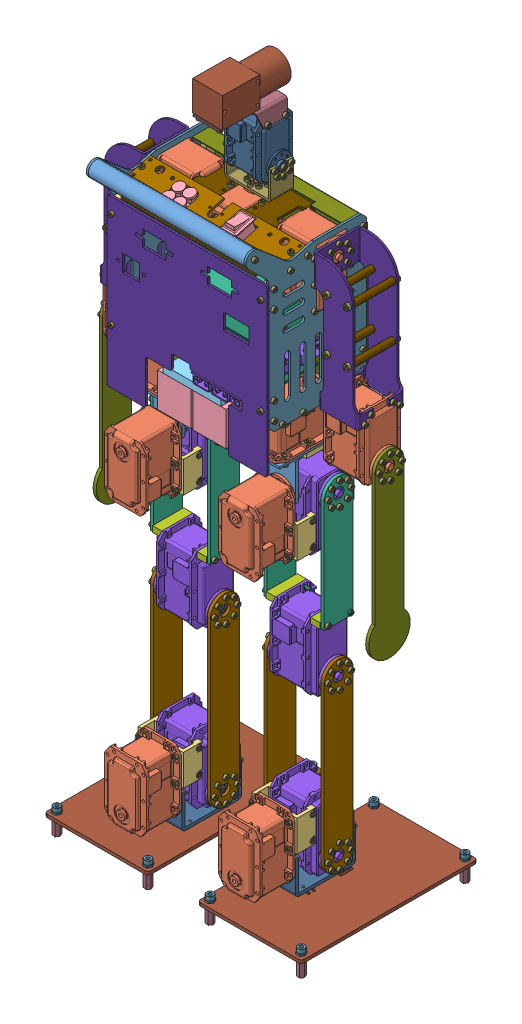
SolidWorks assembly 机器人, configuration 默认. Lengths in mm.
Overall size (525.52 712.77 348.31).
534 component instances, 40 part files, 172 mates.
Components (placement in the parent):
- 右腿-1: 右腿 [默认] at (1333.6429 -132.4302 49.3314) x (0.483512 -0.009844 -0.875282) z (0.842178 0.277849 0.4621) size (197.18 411.3 221.34)
  - 机器人-髋关节连接件-1: 机器人-髋关节连接件 [默认] at (-136.5981 582.4586 -53.7343) x (-0.483512 0.238647 -0.842178) z (-0.875282 -0.142634 0.4621) size (28 38.4 160)
  - MX64-1: MX64 [默认] at (-177.0712 253.729 -123.6615) x (0.483512 -0.238647 0.842178) z (0.875282 0.142634 -0.4621) size (40.2 62.1 50)
  - 机器人-舵机组合件-1: 机器人-舵机组合件 [默认] at (-152.084 293.2165 -100.9324) x (-0.483512 0.238647 -0.842178) z (0.009844 -0.960574 -0.277849) size (7.3 18.5 30)
  - 机器人-舵机组合件-2: 机器人-舵机组合件 [默认] at (-172.8697 274.8043 -145.9868) x (0.483512 -0.238647 0.842178) z (-0.009844 0.960574 0.277849) size (7.3 18.5 30)
  - 机器人-舵盘连接件-1: 机器人-舵盘连接件 [默认] at (-112.2264 257.0796 -159.9407) x (0.483512 -0.238647 0.842178) z (-0.009844 0.960574 0.277849) size (40 11.9 29)
  - MX64虚舵盘-1: MX64虚舵盘 [默认] at (-111.5044 237.7188 -167.2282) x (0.4798 -0.375849 0.792798) z (0.0606 0.915638 0.39741) size (28 4.56 28)
  - 机器人-上腿骨-1: 机器人-上腿骨 [默认] at (-150.3146 558.6458 -87.0655) x (0.483512 -0.238647 0.842178) z (0.875282 0.142634 -0.4621) size (3 122 28)
  - 机器人-上腿骨-2: 机器人-上腿骨 [默认] at (-123.7118 545.5154 -40.7289) x (0.483512 -0.238647 0.842178) z (0.875282 0.142634 -0.4621) size (3 122 28)
  - 机器人-腿骨支撑件-1: 机器人-腿骨支撑件 [默认] at (-147.8304 457.0695 -113.7131) x (0.875282 0.142634 -0.4621) z (0.483512 -0.238647 0.842178) size (30 5.6 9.01)
  - 机器人-腿骨支撑件-2: 机器人-腿骨支撑件 [默认] at (-127.0346 446.8053 -77.491) x (0.875282 0.142634 -0.4621) z (0.483512 -0.238647 0.842178) size (30 5.6 9.01)
  - MX106-2-1: MX106-2 [默认] at (-159.0469 439.041 -156.0263) x (-0.875282 -0.142634 0.4621) z (0.483512 -0.238647 0.842178) size (40.2 65.92 57.58)
  - 机器人-下腿骨-1: 机器人-下腿骨 [默认] at (-148.8152 411.8724 -129.5292) x (-0.875282 -0.142634 0.4621) z (0.483512 -0.238647 0.842178) size (28 178 3)
  - 机器人-下腿骨-2: 机器人-下腿骨 [默认] at (-122.2124 398.742 -83.1925) x (-0.875282 -0.142634 0.4621) z (0.483512 -0.238647 0.842178) size (28 178 3)
  - MX106-2-2: MX106-2 [默认] at (-172.7163 547.584 -117.4089) x (0.875282 0.142634 -0.4621) z (0.483512 -0.238647 0.842178) size (40.2 65.92 57.58)
  - 机器人-舵机组合件-3: 机器人-舵机组合件 [默认] at (-154.489 528.3628 -32.9066) x (-0.483512 0.238647 -0.842178) z (0.009844 -0.960574 -0.277849) size (7.3 18.5 30)
  - 机器人-舵机组合件-4: 机器人-舵机组合件 [默认] at (-175.2748 509.9505 -77.961) x (0.483512 -0.238647 0.842178) z (-0.009844 0.960574 0.277849) size (7.3 18.5 30)
  - MX64-2: MX64 [默认] at (-180.0472 544.5885 -39.5205) x (-0.483512 0.238647 -0.842178) z (0.875282 0.142634 -0.4621) size (40.2 62.1 50)
  - 机器人-舵盘连接件-2: 机器人-舵盘连接件 [默认] at (-115.3502 562.3477 -71.632) x (-0.483512 0.238647 -0.842178) z (0.009844 -0.960574 -0.277849) size (40 11.9 29)
  - MX64虚舵盘-2: MX64虚舵盘 [默认] at (-113.2858 527.9944 -81.0046) x (0.483266 -0.294119 0.824589) z (0.018298 0.945066 0.326368) size (28 4.56 28)
  - MX106-2-3: MX106-2 [默认] at (-157.5702 294.9548 -197.7036) x (-0.875282 -0.142634 0.4621) z (0.483512 -0.238647 0.842178) size (40.2 65.92 57.58)
  - 机器人-踝关节连接件-1: 机器人-踝关节连接件 [默认] at (-133.0412 234.9252 -154.2684) x (0.483512 -0.238647 0.842178) z (-0.875282 -0.142634 0.4621) size (28 33 160)
  - 机器人-脚板-1: 机器人-脚板 [默认] at (-115.9474 228.7929 -143.2594) x (-0.875282 -0.142634 0.4621) z (0.483512 -0.238647 0.842178) size (170 3 100)
  - hexagon socket head cap screws gb-1: hexagon socket head cap screws gb [GB_FASTENER_SCREWS_HSHCS M2.5X6-N] at (-151.4151 548.6761 -92.2273) x (0.483512 -0.238647 0.842178) z (-0.842178 0.135478 0.521902) size (8.5 4.5 4.5)
  - hexagon socket head cap screws gb-2: hexagon socket head cap screws gb [GB_FASTENER_SCREWS_HSHCS M2.5X6-N] at (-144.6387 552.8803 -94.9264) x (0.483512 -0.238647 0.842178) z (-0.842178 0.135478 0.521902) size (8.5 4.5 4.5)
  - hexagon socket head cap screws gb-3: hexagon socket head cap screws gb [GB_FASTENER_SCREWS_HSHCS M2.5X6-N] at (-141.8953 560.8114 -94.254) x (0.483512 -0.238647 0.842178) z (-0.842178 0.135478 0.521902) size (8.5 4.5 4.5)
  - hexagon socket head cap screws gb-4: hexagon socket head cap screws gb [GB_FASTENER_SCREWS_HSHCS M2.5X6-N] at (-144.7919 567.8233 -90.6041) x (0.483512 -0.238647 0.842178) z (-0.842178 0.135478 0.521902) size (8.5 4.5 4.5)
  - hexagon socket head cap screws gb-5: hexagon socket head cap screws gb [GB_FASTENER_SCREWS_HSHCS M2.5X6-N] at (-151.6317 569.8087 -86.1146) x (0.483512 -0.238647 0.842178) z (-0.842178 0.135478 0.521902) size (8.5 4.5 4.5)
  - hexagon socket head cap screws gb-6: hexagon socket head cap screws gb [GB_FASTENER_SCREWS_HSHCS M2.5X6-N] at (-158.4081 565.6045 -83.4155) x (0.483512 -0.238647 0.842178) z (-0.842178 0.135478 0.521902) size (8.5 4.5 4.5)
  - hexagon socket head cap screws gb-7: hexagon socket head cap screws gb [GB_FASTENER_SCREWS_HSHCS M2.5X6-N] at (-161.1515 557.6734 -84.0878) x (0.483512 -0.238647 0.842178) z (-0.842178 0.135478 0.521902) size (8.5 4.5 4.5)
  - hexagon socket head cap screws gb-8: hexagon socket head cap screws gb [GB_FASTENER_SCREWS_HSHCS M2.5X6-N] at (-158.2549 550.6614 -87.7378) x (0.483512 -0.238647 0.842178) z (-0.842178 0.135478 0.521902) size (8.5 4.5 4.5)
  - hexagon socket head cap screws gb-9: hexagon socket head cap screws gb [GB_FASTENER_SCREWS_HSHCS M2.5X6-N] at (-150.1323 423.0353 -128.5783) x (0.483512 -0.238647 0.842178) z (-0.842178 0.135478 0.521902) size (8.5 4.5 4.5)
  - hexagon socket head cap screws gb-10: hexagon socket head cap screws gb [GB_FASTENER_SCREWS_HSHCS M2.5X6-N] at (-143.2925 421.0499 -133.0678) x (0.483512 -0.238647 0.842178) z (-0.842178 0.135478 0.521902) size (8.5 4.5 4.5)
  - hexagon socket head cap screws gb-11: hexagon socket head cap screws gb [GB_FASTENER_SCREWS_HSHCS M2.5X6-N] at (-140.3959 414.038 -136.7177) x (0.483512 -0.238647 0.842178) z (-0.842178 0.135478 0.521902) size (8.5 4.5 4.5)
  - hexagon socket head cap screws gb-12: hexagon socket head cap screws gb [GB_FASTENER_SCREWS_HSHCS M2.5X6-N] at (-143.1393 406.1069 -137.3901) x (0.483512 -0.238647 0.842178) z (-0.842178 0.135478 0.521902) size (8.5 4.5 4.5)
  - hexagon socket head cap screws gb-13: hexagon socket head cap screws gb [GB_FASTENER_SCREWS_HSHCS M2.5X6-N] at (-149.9157 401.9027 -134.691) x (0.483512 -0.238647 0.842178) z (-0.842178 0.135478 0.521902) size (8.5 4.5 4.5)
  - hexagon socket head cap screws gb-14: hexagon socket head cap screws gb [GB_FASTENER_SCREWS_HSHCS M2.5X6-N] at (-159.6521 410.9 -126.5515) x (0.483512 -0.238647 0.842178) z (-0.842178 0.135478 0.521902) size (8.5 4.5 4.5)
  - hexagon socket head cap screws gb-15: hexagon socket head cap screws gb [GB_FASTENER_SCREWS_HSHCS M2.5X6-N] at (-156.7555 403.888 -130.2015) x (0.483512 -0.238647 0.842178) z (-0.842178 0.135478 0.521902) size (8.5 4.5 4.5)
  - hexagon socket head cap screws gb-16: hexagon socket head cap screws gb [GB_FASTENER_SCREWS_HSHCS M2.5X6-N] at (-156.9087 418.8311 -125.8792) x (0.483512 -0.238647 0.842178) z (-0.842178 0.135478 0.521902) size (8.5 4.5 4.5)
  - hexagon socket head cap screws gb-17: hexagon socket head cap screws gb [GB_FASTENER_SCREWS_HSHCS M2.5X6-N] at (-141.6627 262.0207 -179.0674) x (0.483512 -0.238647 0.842178) z (-0.842178 0.135478 0.521902) size (8.5 4.5 4.5)
  - hexagon socket head cap screws gb-18: hexagon socket head cap screws gb [GB_FASTENER_SCREWS_HSHCS M2.5X6-N] at (-148.4391 257.8165 -176.3683) x (0.483512 -0.238647 0.842178) z (-0.842178 0.135478 0.521902) size (8.5 4.5 4.5)
  - hexagon socket head cap screws gb-19: hexagon socket head cap screws gb [GB_FASTENER_SCREWS_HSHCS M2.5X6-N] at (-155.2789 259.8019 -171.8788) x (0.483512 -0.238647 0.842178) z (-0.842178 0.135478 0.521902) size (8.5 4.5 4.5)
  - hexagon socket head cap screws gb-20: hexagon socket head cap screws gb [GB_FASTENER_SCREWS_HSHCS M2.5X6-N] at (-158.1755 266.8139 -168.2288) x (0.483512 -0.238647 0.842178) z (-0.842178 0.135478 0.521902) size (8.5 4.5 4.5)
  - hexagon socket head cap screws gb-21: hexagon socket head cap screws gb [GB_FASTENER_SCREWS_HSHCS M2.5X6-N] at (-138.9192 269.9518 -178.395) x (0.483512 -0.238647 0.842178) z (-0.842178 0.135478 0.521902) size (8.5 4.5 4.5)
  - hexagon socket head cap screws gb-22: hexagon socket head cap screws gb [GB_FASTENER_SCREWS_HSHCS M2.5X6-N] at (-141.8158 276.9638 -174.7451) x (0.483512 -0.238647 0.842178) z (-0.842178 0.135478 0.521902) size (8.5 4.5 4.5)
  - hexagon socket head cap screws gb-23: hexagon socket head cap screws gb [GB_FASTENER_SCREWS_HSHCS M2.5X6-N] at (-148.6556 278.9491 -170.2556) x (0.483512 -0.238647 0.842178) z (-0.842178 0.135478 0.521902) size (8.5 4.5 4.5)
  - hexagon socket head cap screws gb-24: hexagon socket head cap screws gb [GB_FASTENER_SCREWS_HSHCS M2.5X6-N] at (-155.432 274.7449 -167.5565) x (0.483512 -0.238647 0.842178) z (-0.842178 0.135478 0.521902) size (8.5 4.5 4.5)
  - hexagon socket head cap screws gb-25: hexagon socket head cap screws gb [GB_FASTENER_SCREWS_HSHCS M2.5X6-N] at (-175.1097 276.8595 -138.7751) x (0.875282 0.142634 -0.4621) z (0.4621 0.035147 0.886131) size (8.5 4.5 4.5)
  - hexagon socket head cap screws gb-26: hexagon socket head cap screws gb [GB_FASTENER_SCREWS_HSHCS M2.5X6-N] at (-175.3263 297.9922 -132.6624) x (0.875282 0.142634 -0.4621) z (0.4621 0.035147 0.886131) size (8.5 4.5 4.5)
  - hexagon socket head cap screws gb-27: hexagon socket head cap screws gb [GB_FASTENER_SCREWS_HSHCS M2.5X6-N] at (-151.5797 247.299 -140.1187) x (-0.875282 -0.142634 0.4621) z (-0.4621 0.528483 -0.712158) size (8.5 4.5 4.5)
  - hexagon socket head cap screws gb-28: hexagon socket head cap screws gb [GB_FASTENER_SCREWS_HSHCS M2.5X6-N] at (-155.3722 252.2501 -145.7741) x (-0.875282 -0.142634 0.4621) z (-0.4621 0.528483 -0.712158) size (8.5 4.5 4.5)
  - hexagon socket head cap screws gb-31: hexagon socket head cap screws gb [GB_FASTENER_SCREWS_HSHCS M2.5X6-N] at (-157.0066 260.4905 -146.3263) x (-0.875282 -0.142634 0.4621) z (-0.4621 0.528483 -0.712158) size (8.5 4.5 4.5)
  - hexagon socket head cap screws gb-34: hexagon socket head cap screws gb [GB_FASTENER_SCREWS_HSHCS M2.5X6-N] at (-154.7723 559.2912 -49.865) x (-0.875282 -0.142634 0.4621) z (-0.4621 0.528483 -0.712158) size (8.5 4.5 4.5)
  - hexagon socket head cap screws gb-35: hexagon socket head cap screws gb [GB_FASTENER_SCREWS_HSHCS M2.5X6-N] at (-158.5014 558.0527 -57.3108) x (-0.875282 -0.142634 0.4621) z (-0.4621 0.528483 -0.712158) size (8.5 4.5 4.5)
  - hexagon socket head cap screws gb-36: hexagon socket head cap screws gb [GB_FASTENER_SCREWS_HSHCS M2.5X6-N] at (-159.9827 551.35 -62.1853) x (-0.875282 -0.142634 0.4621) z (-0.4621 0.528483 -0.712158) size (8.5 4.5 4.5)
  - hexagon socket head cap screws gb-37: hexagon socket head cap screws gb [GB_FASTENER_SCREWS_HSHCS M2.5X6-N] at (-177.7314 533.1384 -64.6366) x (0.875282 0.142634 -0.4621) z (0.4621 0.035147 0.886131) size (8.5 4.5 4.5)
  - hexagon socket head cap screws gb-38: hexagon socket head cap screws gb [GB_FASTENER_SCREWS_HSHCS M2.5X6-N] at (-177.5148 512.0058 -70.7493) x (0.875282 0.142634 -0.4621) z (0.4621 0.035147 0.886131) size (8.5 4.5 4.5)
  - hexagon socket head cap screws gb-39: hexagon socket head cap screws gb [GB_FASTENER_SCREWS_HSHCS M2.5X6-N] at (-121.1608 554.7692 -33.0405) x (-0.483512 0.238647 -0.842178) z (0.842178 0.389134 -0.373244) size (8.5 4.5 4.5)
  - hexagon socket head cap screws gb-40: hexagon socket head cap screws gb [GB_FASTENER_SCREWS_HSHCS M2.5X6-N] at (-127.9371 550.5649 -30.3414) x (-0.483512 0.238647 -0.842178) z (0.842178 0.389134 -0.373244) size (8.5 4.5 4.5)
  - hexagon socket head cap screws gb-41: hexagon socket head cap screws gb [GB_FASTENER_SCREWS_HSHCS M2.5X6-N] at (-130.6806 542.6339 -31.0138) x (-0.483512 0.238647 -0.842178) z (0.842178 0.389134 -0.373244) size (8.5 4.5 4.5)
  - hexagon socket head cap screws gb-42: hexagon socket head cap screws gb [GB_FASTENER_SCREWS_HSHCS M2.5X6-N] at (-127.784 535.6219 -34.6637) x (-0.483512 0.238647 -0.842178) z (0.842178 0.389134 -0.373244) size (8.5 4.5 4.5)
  - hexagon socket head cap screws gb-43: hexagon socket head cap screws gb [GB_FASTENER_SCREWS_HSHCS M2.5X6-N] at (-120.9442 533.6365 -39.1532) x (-0.483512 0.238647 -0.842178) z (0.842178 0.389134 -0.373244) size (8.5 4.5 4.5)
  - hexagon socket head cap screws gb-44: hexagon socket head cap screws gb [GB_FASTENER_SCREWS_HSHCS M2.5X6-N] at (-114.1678 537.8408 -41.8523) x (-0.483512 0.238647 -0.842178) z (0.842178 0.389134 -0.373244) size (8.5 4.5 4.5)
  - hexagon socket head cap screws gb-45: hexagon socket head cap screws gb [GB_FASTENER_SCREWS_HSHCS M2.5X6-N] at (-111.4244 545.7718 -41.18) x (-0.483512 0.238647 -0.842178) z (0.842178 0.389134 -0.373244) size (8.5 4.5 4.5)
  - hexagon socket head cap screws gb-46: hexagon socket head cap screws gb [GB_FASTENER_SCREWS_HSHCS M2.5X6-N] at (-114.3209 552.7838 -37.53) x (-0.483512 0.238647 -0.842178) z (0.842178 0.389134 -0.373244) size (8.5 4.5 4.5)
  - hexagon socket head cap screws gb-47: hexagon socket head cap screws gb [GB_FASTENER_SCREWS_HSHCS M2.5X6-N] at (-106.8769 567.0962 -75.1512) x (-0.875282 -0.142634 0.4621) z (-0.4621 0.528483 -0.712158) size (8.5 4.5 4.5)
  - hexagon socket head cap screws gb-48: hexagon socket head cap screws gb [GB_FASTENER_SCREWS_HSHCS M2.5X6-N] at (-103.0843 562.1451 -69.4957) x (-0.875282 -0.142634 0.4621) z (-0.4621 0.528483 -0.712158) size (8.5 4.5 4.5)
  - hexagon socket head cap screws gb-49: hexagon socket head cap screws gb [GB_FASTENER_SCREWS_HSHCS M2.5X6-N] at (-110.606 565.8576 -82.5969) x (-0.875282 -0.142634 0.4621) z (-0.4621 0.528483 -0.712158) size (8.5 4.5 4.5)
  - hexagon socket head cap screws gb-50: hexagon socket head cap screws gb [GB_FASTENER_SCREWS_HSHCS M2.5X6-N] at (-101.4499 553.9047 -68.9435) x (-0.875282 -0.142634 0.4621) z (-0.4621 0.528483 -0.712158) size (8.5 4.5 4.5)
  - hexagon socket head cap screws gb-51: hexagon socket head cap screws gb [GB_FASTENER_SCREWS_HSHCS M2.5X6-N] at (-112.0872 559.155 -87.4714) x (-0.875282 -0.142634 0.4621) z (-0.4621 0.528483 -0.712158) size (8.5 4.5 4.5)
  - hexagon socket head cap screws gb-55: hexagon socket head cap screws gb [GB_FASTENER_SCREWS_HSHCS M2.5X6-N] at (-150.9798 554.3402 -44.2096) x (-0.875282 -0.142634 0.4621) z (-0.4621 0.528483 -0.712158) size (8.5 4.5 4.5)
  - hexagon socket head cap screws gb-56: hexagon socket head cap screws gb [GB_FASTENER_SCREWS_HSHCS M2.5X6-N] at (-149.3454 546.0998 -43.6574) x (-0.875282 -0.142634 0.4621) z (-0.4621 0.528483 -0.712158) size (8.5 4.5 4.5)
  - hexagon socket head cap screws gb-58: hexagon socket head cap screws gb [GB_FASTENER_SCREWS_HSHCS M2.5X6-N] at (-161.0019 524.8812 -35.4973) x (0.875282 0.142634 -0.4621) z (0.4621 0.035147 0.886131) size (8.5 4.5 4.5)
  - hexagon socket head cap screws gb-59: hexagon socket head cap screws gb [GB_FASTENER_SCREWS_HSHCS M2.5X6-N] at (-160.7853 503.7486 -41.6099) x (0.875282 0.142634 -0.4621) z (0.4621 0.035147 0.886131) size (8.5 4.5 4.5)
  - hexagon socket head cap screws gb-60: hexagon socket head cap screws gb [GB_FASTENER_SCREWS_HSHCS M2.5X6-N] at (-119.6614 407.9958 -75.5042) x (-0.483512 0.238647 -0.842178) z (0.842178 0.389134 -0.373244) size (8.5 4.5 4.5)
  - hexagon socket head cap screws gb-61: hexagon socket head cap screws gb [GB_FASTENER_SCREWS_HSHCS M2.5X6-N] at (-126.4377 403.7915 -72.8051) x (-0.483512 0.238647 -0.842178) z (0.842178 0.389134 -0.373244) size (8.5 4.5 4.5)
  - hexagon socket head cap screws gb-62: hexagon socket head cap screws gb [GB_FASTENER_SCREWS_HSHCS M2.5X6-N] at (-129.1812 395.8605 -73.4775) x (-0.483512 0.238647 -0.842178) z (0.842178 0.389134 -0.373244) size (8.5 4.5 4.5)
  - hexagon socket head cap screws gb-63: hexagon socket head cap screws gb [GB_FASTENER_SCREWS_HSHCS M2.5X6-N] at (-126.2846 388.8485 -77.1274) x (-0.483512 0.238647 -0.842178) z (0.842178 0.389134 -0.373244) size (8.5 4.5 4.5)
  - hexagon socket head cap screws gb-64: hexagon socket head cap screws gb [GB_FASTENER_SCREWS_HSHCS M2.5X6-N] at (-119.4448 386.8631 -81.6169) x (-0.483512 0.238647 -0.842178) z (0.842178 0.389134 -0.373244) size (8.5 4.5 4.5)
  - hexagon socket head cap screws gb-65: hexagon socket head cap screws gb [GB_FASTENER_SCREWS_HSHCS M2.5X6-N] at (-112.6684 391.0674 -84.316) x (-0.483512 0.238647 -0.842178) z (0.842178 0.389134 -0.373244) size (8.5 4.5 4.5)
  - hexagon socket head cap screws gb-66: hexagon socket head cap screws gb [GB_FASTENER_SCREWS_HSHCS M2.5X6-N] at (-109.925 398.9984 -83.6437) x (-0.483512 0.238647 -0.842178) z (0.842178 0.389134 -0.373244) size (8.5 4.5 4.5)
  - hexagon socket head cap screws gb-67: hexagon socket head cap screws gb [GB_FASTENER_SCREWS_HSHCS M2.5X6-N] at (-112.8216 406.0104 -79.9937) x (-0.483512 0.238647 -0.842178) z (0.842178 0.389134 -0.373244) size (8.5 4.5 4.5)
  - hexagon socket head cap screws gb-68: hexagon socket head cap screws gb [GB_FASTENER_SCREWS_HSHCS M2.5X6-N] at (-158.5968 289.735 -103.523) x (0.875282 0.142634 -0.4621) z (0.4621 0.035147 0.886131) size (8.5 4.5 4.5)
  - hexagon socket head cap screws gb-69: hexagon socket head cap screws gb [GB_FASTENER_SCREWS_HSHCS M2.5X6-N] at (-158.3802 268.6023 -109.6357) x (0.875282 0.142634 -0.4621) z (0.4621 0.035147 0.886131) size (8.5 4.5 4.5)
  - hexagon socket head cap screws gb-70: hexagon socket head cap screws gb [GB_FASTENER_SCREWS_HSHCS M2.5X6-N] at (-118.1847 263.9096 -117.1815) x (-0.483512 0.238647 -0.842178) z (0.842178 0.389134 -0.373244) size (8.5 4.5 4.5)
  - hexagon socket head cap screws gb-71: hexagon socket head cap screws gb [GB_FASTENER_SCREWS_HSHCS M2.5X6-N] at (-124.9611 259.7054 -114.4824) x (-0.483512 0.238647 -0.842178) z (0.842178 0.389134 -0.373244) size (8.5 4.5 4.5)
  - hexagon socket head cap screws gb-72: hexagon socket head cap screws gb [GB_FASTENER_SCREWS_HSHCS M2.5X6-N] at (-127.7045 251.7743 -115.1548) x (-0.483512 0.238647 -0.842178) z (0.842178 0.389134 -0.373244) size (8.5 4.5 4.5)
  - hexagon socket head cap screws gb-73: hexagon socket head cap screws gb [GB_FASTENER_SCREWS_HSHCS M2.5X6-N] at (-124.8079 244.7624 -118.8047) x (-0.483512 0.238647 -0.842178) z (0.842178 0.389134 -0.373244) size (8.5 4.5 4.5)
  - hexagon socket head cap screws gb-74: hexagon socket head cap screws gb [GB_FASTENER_SCREWS_HSHCS M2.5X6-N] at (-117.9681 242.777 -123.2942) x (-0.483512 0.238647 -0.842178) z (0.842178 0.389134 -0.373244) size (8.5 4.5 4.5)
  - hexagon socket head cap screws gb-75: hexagon socket head cap screws gb [GB_FASTENER_SCREWS_HSHCS M2.5X6-N] at (-111.1917 246.9812 -125.9933) x (-0.483512 0.238647 -0.842178) z (0.842178 0.389134 -0.373244) size (8.5 4.5 4.5)
  - hexagon socket head cap screws gb-76: hexagon socket head cap screws gb [GB_FASTENER_SCREWS_HSHCS M2.5X6-N] at (-108.4483 254.9123 -125.321) x (-0.483512 0.238647 -0.842178) z (0.842178 0.389134 -0.373244) size (8.5 4.5 4.5)
  - hexagon socket head cap screws gb-77: hexagon socket head cap screws gb [GB_FASTENER_SCREWS_HSHCS M2.5X6-N] at (-111.3449 261.9242 -121.671) x (-0.483512 0.238647 -0.842178) z (0.842178 0.389134 -0.373244) size (8.5 4.5 4.5)
  - hexagon socket head cap screws gb-79: hexagon socket head cap screws gb [GB_FASTENER_SCREWS_HSHCS M2.5X6-N] at (-146.3693 255.2403 -127.7984) x (-0.875282 -0.142634 0.4621) z (-0.4621 0.528483 -0.712158) size (8.5 4.5 4.5)
  - hexagon socket head cap screws gb-80: hexagon socket head cap screws gb [GB_FASTENER_SCREWS_HSHCS M2.5X6-N] at (-147.8506 248.5376 -132.6729) x (-0.875282 -0.142634 0.4621) z (-0.4621 0.528483 -0.712158) size (8.5 4.5 4.5)
  - hexagon socket head cap screws gb-84: hexagon socket head cap screws gb [GB_FASTENER_SCREWS_HSHCS M2.5X6-N] at (-109.1112 268.2954 -171.6124) x (-0.875282 -0.142634 0.4621) z (-0.4621 0.528483 -0.712158) size (8.5 4.5 4.5)
  - hexagon socket head cap screws gb-85: hexagon socket head cap screws gb [GB_FASTENER_SCREWS_HSHCS M2.5X6-N] at (-107.4768 260.055 -171.0602) x (-0.875282 -0.142634 0.4621) z (-0.4621 0.528483 -0.712158) size (8.5 4.5 4.5)
  - hexagon socket head cap screws gb-86: hexagon socket head cap screws gb [GB_FASTENER_SCREWS_HSHCS M2.5X6-N] at (-98.4739 263.0452 -153.0845) x (-0.875282 -0.142634 0.4621) z (-0.4621 0.528483 -0.712158) size (8.5 4.5 4.5)
  - hexagon socket head cap screws gb-87: hexagon socket head cap screws gb [GB_FASTENER_SCREWS_HSHCS M2.5X6-N] at (-99.9551 256.3425 -157.959) x (-0.875282 -0.142634 0.4621) z (-0.4621 0.528483 -0.712158) size (8.5 4.5 4.5)
  - hexagon socket head cap screws gb-88: hexagon socket head cap screws gb [GB_FASTENER_SCREWS_HSHCS M2.5X6-N] at (-103.6842 255.104 -165.4048) x (-0.875282 -0.142634 0.4621) z (-0.4621 0.528483 -0.712158) size (8.5 4.5 4.5)
  - hexagon socket head cap screws gb-89: hexagon socket head cap screws gb [GB_FASTENER_SCREWS_HSHCS M2.5X6-N] at (-141.6435 221.853 -139.9725) x (-0.009844 0.960574 0.277849) z (-0.277849 -0.269548 0.922033) size (8.5 4.5 4.5)
  - hexagon socket head cap screws gb-90: hexagon socket head cap screws gb [GB_FASTENER_SCREWS_HSHCS M2.5X6-N] at (-152.2807 227.1033 -158.5005) x (-0.009844 0.960574 0.277849) z (-0.277849 -0.269548 0.922033) size (8.5 4.5 4.5)
  - hexagon socket head cap screws gb-91: hexagon socket head cap screws gb [GB_FASTENER_SCREWS_HSHCS M2.5X6-N] at (-124.2717 231.6675 -173.2877) x (-0.009844 0.960574 0.277849) z (-0.277849 -0.269548 0.922033) size (8.5 4.5 4.5)
  - hexagon socket head cap screws gb-92: hexagon socket head cap screws gb [GB_FASTENER_SCREWS_HSHCS M2.5X6-N] at (-113.6344 226.4173 -154.7597) x (-0.009844 0.960574 0.277849) z (-0.277849 -0.269548 0.922033) size (8.5 4.5 4.5)
  - hexagon socket head cap screws gb-93: hexagon socket head cap screws gb [GB_FASTENER_SCREWS_HSHCS M2.5X6-N] at (-129.0043 264.8555 -174.8212) x (0.483512 -0.238647 0.842178) z (-0.842178 0.135478 0.521902) size (8.5 4.5 4.5)
  - hexagon socket head cap screws gb-94: hexagon socket head cap screws gb [GB_FASTENER_SCREWS_HSHCS M2.5X6-N] at (-129.2209 285.9881 -168.7085) x (0.483512 -0.238647 0.842178) z (-0.842178 0.135478 0.521902) size (8.5 4.5 4.5)
  - hexagon socket head cap screws gb-95: hexagon socket head cap screws gb [GB_FASTENER_SCREWS_HSHCS M2.5X6-N] at (-159.409 281.0053 -152.5514) x (0.483512 -0.238647 0.842178) z (-0.842178 0.135478 0.521902) size (8.5 4.5 4.5)
  - hexagon socket head cap screws gb-96: hexagon socket head cap screws gb [GB_FASTENER_SCREWS_HSHCS M2.5X6-N] at (-159.6255 302.1379 -146.4388) x (0.483512 -0.238647 0.842178) z (-0.842178 0.135478 0.521902) size (8.5 4.5 4.5)
  - hexagon socket head cap screws gb-97: hexagon socket head cap screws gb [GB_FASTENER_SCREWS_HSHCS M2.5X6-N] at (-107.4628 275.249 -130.8105) x (-0.483512 0.238647 -0.842178) z (0.842178 0.389134 -0.373244) size (8.5 4.5 4.5)
  - hexagon socket head cap screws gb-98: hexagon socket head cap screws gb [GB_FASTENER_SCREWS_HSHCS M2.5X6-N] at (-107.2463 254.1164 -136.9232) x (-0.483512 0.238647 -0.842178) z (0.842178 0.389134 -0.373244) size (8.5 4.5 4.5)
  - hexagon socket head cap screws gb-99: hexagon socket head cap screws gb [GB_FASTENER_SCREWS_HSHCS M2.5X6-N] at (-138.0609 291.4943 -108.8776) x (-0.483512 0.238647 -0.842178) z (0.842178 0.389134 -0.373244) size (8.5 4.5 4.5)
  - hexagon socket head cap screws gb-100: hexagon socket head cap screws gb [GB_FASTENER_SCREWS_HSHCS M2.5X6-N] at (-137.8443 270.3616 -114.9903) x (-0.483512 0.238647 -0.842178) z (0.842178 0.389134 -0.373244) size (8.5 4.5 4.5)
  - hexagon socket head cap screws gb-101: hexagon socket head cap screws gb [GB_FASTENER_SCREWS_HSHCS M2.5X6-N] at (-140.466 526.6405 -40.8519) x (-0.483512 0.238647 -0.842178) z (0.842178 0.389134 -0.373244) size (8.5 4.5 4.5)
  - hexagon socket head cap screws gb-102: hexagon socket head cap screws gb [GB_FASTENER_SCREWS_HSHCS M2.5X6-N] at (-140.2494 505.5079 -46.9645) x (-0.483512 0.238647 -0.842178) z (0.842178 0.389134 -0.373244) size (8.5 4.5 4.5)
  - hexagon socket head cap screws gb-103: hexagon socket head cap screws gb [GB_FASTENER_SCREWS_HSHCS M2.5X6-N] at (-110.3011 552.6605 -50.5594) x (-0.483512 0.238647 -0.842178) z (0.842178 0.389134 -0.373244) size (8.5 4.5 4.5)
  - hexagon socket head cap screws gb-104: hexagon socket head cap screws gb [GB_FASTENER_SCREWS_HSHCS M2.5X6-N] at (-110.0845 531.5279 -56.6721) x (-0.483512 0.238647 -0.842178) z (0.842178 0.389134 -0.373244) size (8.5 4.5 4.5)
  - hexagon socket head cap screws gb-105: hexagon socket head cap screws gb [GB_FASTENER_SCREWS_HSHCS M2.5X6-N] at (-162.0306 537.2841 -78.413) x (0.483512 -0.238647 0.842178) z (-0.842178 0.135478 0.521902) size (8.5 4.5 4.5)
  - hexagon socket head cap screws gb-106: hexagon socket head cap screws gb [GB_FASTENER_SCREWS_HSHCS M2.5X6-N] at (-161.814 516.1515 -84.5257) x (0.483512 -0.238647 0.842178) z (-0.842178 0.135478 0.521902) size (8.5 4.5 4.5)
  - hexagon socket head cap screws gb-107: hexagon socket head cap screws gb [GB_FASTENER_SCREWS_HSHCS M2.5X6-N] at (-131.8425 542.267 -94.5701) x (0.483512 -0.238647 0.842178) z (-0.842178 0.135478 0.521902) size (8.5 4.5 4.5)
  - hexagon socket head cap screws gb-108: hexagon socket head cap screws gb [GB_FASTENER_SCREWS_HSHCS M2.5X6-N] at (-132.0591 563.3996 -88.4574) x (0.483512 -0.238647 0.842178) z (-0.842178 0.135478 0.521902) size (8.5 4.5 4.5)
  - hexagon socket head cap screws gb-110: hexagon socket head cap screws gb [GB_FASTENER_SCREWS_HSHCS M2.5X6-N] at (-160.1178 456.8131 -113.2619) x (0.483512 -0.238647 0.842178) z (-0.842178 0.135478 0.521902) size (8.5 4.5 4.5)
  - hexagon socket head cap screws gb-111: hexagon socket head cap screws gb [GB_FASTENER_SCREWS_HSHCS M2.5X6-N] at (-129.6469 441.7736 -60.1879) x (-0.483512 0.238647 -0.842178) z (0.842178 0.389134 -0.373244) size (8.5 4.5 4.5)
  - hexagon socket head cap screws gb-115: hexagon socket head cap screws gb [GB_FASTENER_SCREWS_HSHCS M2.5X6-N] at (-109.7795 556.0392 -76.6179) x (-0.875282 -0.142634 0.4621) z (-0.4621 0.528483 -0.712158) size (8.5 4.5 4.5)
  - hexagon socket head cap screws gb-116: hexagon socket head cap screws gb [GB_FASTENER_SCREWS_HSHCS M2.5X6-N] at (-149.8601 558.4214 -86.2738) x (0.483512 -0.238647 0.842178) z (-0.842178 0.135478 0.521902) size (8.5 4.5 4.5)
  - hexagon socket head cap screws gb-117: hexagon socket head cap screws gb [GB_FASTENER_SCREWS_HSHCS M2.5X6-N] at (-148.3607 411.648 -128.7375) x (0.483512 -0.238647 0.842178) z (-0.842178 0.135478 0.521902) size (8.5 4.5 4.5)
  - hexagon socket head cap screws gb-118: hexagon socket head cap screws gb [GB_FASTENER_SCREWS_HSHCS M2.5X6-N] at (-146.8841 267.5619 -170.4148) x (0.483512 -0.238647 0.842178) z (-0.842178 0.135478 0.521902) size (8.5 4.5 4.5)
  - hexagon socket head cap screws gb-119: hexagon socket head cap screws gb [GB_FASTENER_SCREWS_HSHCS M2.5X6-N] at (-106.8035 265.1796 -160.7589) x (-0.875282 -0.142634 0.4621) z (-0.4621 0.528483 -0.712158) size (8.5 4.5 4.5)
  - 脚钉铜柱-1: 脚钉铜柱 [默认] at (-163.643 189.734 -74.699) x (0.999951 0.009844 0.001395) z (0.001395 -0.277849 0.960624) size (6.82 21 6.51)
  - 脚钉铜柱-2: 脚钉铜柱 [默认] at (-25.3484 212.2701 -147.7108) x (0.999951 0.009844 0.001395) z (0.001395 -0.277849 0.960624) size (6.82 21 6.51)
  - 脚钉铜柱-3: 脚钉铜柱 [默认] at (-67.8975 233.2711 -221.8225) x (0.999951 0.009844 0.001395) z (0.001395 -0.277849 0.960624) size (6.82 21 6.51)
  - 脚钉铜柱-4: 脚钉铜柱 [默认] at (-206.1921 210.7349 -148.8107) x (0.999951 0.009844 0.001395) z (0.001395 -0.277849 0.960624) size (6.82 21 6.51)
  - prevailing torque type style 1 gb-1: prevailing torque type style 1 gb [GB_HEXAGON_TYPE9 M4-N] at (-68.0975 252.7899 -216.1766) x (0.999924 0.0074 0.009844) z (-0.009844 0.960574 0.277849) size (8.08 7 6)
  - prevailing torque type style 1 gb-2: prevailing torque type style 1 gb [GB_HEXAGON_TYPE9 M4-N] at (-25.5485 231.789 -142.0649) x (0.999924 0.0074 0.009844) z (-0.009844 0.960574 0.277849) size (8.08 7 6)
  - prevailing torque type style 1 gb-3: prevailing torque type style 1 gb [GB_HEXAGON_TYPE9 M4-N] at (-206.3921 230.2538 -143.1648) x (0.999924 0.0074 0.009844) z (-0.009844 0.960574 0.277849) size (8.08 7 6)
  - prevailing torque type style 1 gb-4: prevailing torque type style 1 gb [GB_HEXAGON_TYPE9 M4-N] at (-163.8431 209.2529 -69.0531) x (0.999924 0.0074 0.009844) z (-0.009844 0.960574 0.277849) size (8.08 7 6)
  - slotted cheese head screws gb-2: slotted cheese head screws gb [GB_FASTENER_SCREWS_SCHS M2.5X20-20-N] at (-140.5232 459.784 -122.8386) x (0.483512 -0.238647 0.842178) z (-0.842178 0.135478 0.521902) size (21.81 4.5 4.5)
  - slotted cheese head screws gb-3: slotted cheese head screws gb [GB_FASTENER_SCREWS_SCHS M2.5X20-20-N] at (-110.7292 445.0786 -70.9436) x (-0.483512 0.238647 -0.842178) z (0.842178 0.389134 -0.373244) size (21.81 4.5 4.5)
- 左腿-1: 左腿 [默认] at (1223.8429 -132.4302 49.3314) x (0.483512 -0.009844 -0.875282) z (0.842178 0.277849 0.4621) size (197.18 402.23 253.32)
  - 机器人-髋关节连接件-1: 机器人-髋关节连接件 [默认] at (-136.5981 582.4586 -53.7343) x (-0.483512 0.238647 -0.842178) z (-0.875282 -0.142634 0.4621) size (28 38.4 160)
  - MX64-1: MX64 [默认] at (-176.9039 253.7499 -123.7278) x (0.483512 -0.238647 0.842178) z (0.875282 0.142634 -0.4621) size (40.2 62.1 50)
  - 机器人-舵机组合件-1: 机器人-舵机组合件 [默认] at (-151.9167 293.2374 -100.9987) x (-0.483512 0.238647 -0.842178) z (0.009844 -0.960574 -0.277849) size (7.3 18.5 30)
  - 机器人-舵机组合件-2: 机器人-舵机组合件 [默认] at (-172.7025 274.8252 -146.0531) x (0.483512 -0.238647 0.842178) z (-0.009844 0.960574 0.277849) size (7.3 18.5 30)
  - 机器人-舵盘连接件-1: 机器人-舵盘连接件 [默认] at (-112.0592 257.1005 -160.0071) x (0.483512 -0.238647 0.842178) z (-0.009844 0.960574 0.277849) size (40 11.9 29)
  - MX64虚舵盘-1: MX64虚舵盘 [默认] at (-111.4947 237.7141 -167.2113) x (0.4798 -0.375849 0.792798) z (0.0606 0.915638 0.39741) size (28 4.56 28)
  - 机器人-上腿骨-1: 机器人-上腿骨 [默认] at (-150.1474 558.6667 -87.1318) x (0.483512 -0.238647 0.842178) z (0.875282 0.142634 -0.4621) size (3 122 28)
  - 机器人-上腿骨-2: 机器人-上腿骨 [默认] at (-123.5446 545.5363 -40.7952) x (0.483512 -0.238647 0.842178) z (0.875282 0.142634 -0.4621) size (3 122 28)
  - 机器人-腿骨支撑件-1: 机器人-腿骨支撑件 [默认] at (-147.6632 457.0904 -113.7794) x (0.875282 0.142634 -0.4621) z (0.483512 -0.238647 0.842178) size (30 5.6 9.01)
  - 机器人-腿骨支撑件-2: 机器人-腿骨支撑件 [默认] at (-126.8673 446.8262 -77.5573) x (0.875282 0.142634 -0.4621) z (0.483512 -0.238647 0.842178) size (30 5.6 9.01)
  - MX106-2-1: MX106-2 [默认] at (-110.7242 407.0604 -43.7512) x (0.875282 0.142634 -0.4621) z (-0.483512 0.238647 -0.842178) size (40.2 65.92 57.58)
  - 机器人-下腿骨-1: 机器人-下腿骨 [默认] at (-148.6383 411.8885 -129.5787) x (-0.875282 -0.142634 0.4621) z (0.483512 -0.238647 0.842178) size (28 178 3)
  - 机器人-下腿骨-2: 机器人-下腿骨 [默认] at (-122.0355 398.7582 -83.242) x (-0.875282 -0.142634 0.4621) z (0.483512 -0.238647 0.842178) size (28 178 3)
  - MX106-2-2: MX106-2 [默认] at (-99.3215 519.6954 -18.3924) x (-0.875282 -0.142634 0.4621) z (-0.483512 0.238647 -0.842178) size (40.2 65.92 57.58)
  - 机器人-舵机组合件-3: 机器人-舵机组合件 [默认] at (-154.3315 528.3884 -32.9898) x (-0.483512 0.238647 -0.842178) z (0.009844 -0.960574 -0.277849) size (7.3 18.5 30)
  - 机器人-舵机组合件-4: 机器人-舵机组合件 [默认] at (-175.1173 509.9762 -78.0442) x (0.483512 -0.238647 0.842178) z (-0.009844 0.960574 0.277849) size (7.3 18.5 30)
  - MX64-2: MX64 [默认] at (-180.0472 544.5885 -39.5205) x (-0.483512 0.238647 -0.842178) z (0.875282 0.142634 -0.4621) size (40.2 62.1 50)
  - 机器人-舵盘连接件-2: 机器人-舵盘连接件 [默认] at (-115.1926 562.3734 -71.7152) x (-0.483512 0.238647 -0.842178) z (0.009844 -0.960574 -0.277849) size (40 11.9 29)
  - MX64虚舵盘-2: MX64虚舵盘 [默认] at (-113.2858 527.9944 -81.0046) x (0.483266 -0.294119 0.824589) z (0.018298 0.945066 0.326368) size (28 4.56 28)
  - MX106-2-3: MX106-2 [默认] at (-109.2475 262.9742 -85.4285) x (0.875282 0.142634 -0.4621) z (-0.483512 0.238647 -0.842178) size (40.2 65.92 57.58)
  - 机器人-踝关节连接件-1: 机器人-踝关节连接件 [默认] at (-133.0316 234.9204 -154.2515) x (0.483512 -0.238647 0.842178) z (-0.875282 -0.142634 0.4621) size (28 33 160)
  - 机器人-脚板-1: 机器人-脚板 [默认] at (-134.2817 234.9749 -176.0789) x (-0.875282 -0.142634 0.4621) z (-0.483512 0.238647 -0.842178) size (170 3 100)
  - hexagon socket head cap screws gb-1: hexagon socket head cap screws gb [GB_FASTENER_SCREWS_HSHCS M2.5X6-N] at (-103.0843 562.1451 -69.4957) x (-0.875282 -0.142634 0.4621) z (-0.4621 0.528483 -0.712158) size (8.5 4.5 4.5)
  - hexagon socket head cap screws gb-2: hexagon socket head cap screws gb [GB_FASTENER_SCREWS_HSHCS M2.5X6-N] at (-110.606 565.8576 -82.5969) x (-0.875282 -0.142634 0.4621) z (-0.4621 0.528483 -0.712158) size (8.5 4.5 4.5)
  - hexagon socket head cap screws gb-3: hexagon socket head cap screws gb [GB_FASTENER_SCREWS_HSHCS M2.5X6-N] at (-106.8769 567.0962 -75.1512) x (-0.875282 -0.142634 0.4621) z (-0.4621 0.528483 -0.712158) size (8.5 4.5 4.5)
  - hexagon socket head cap screws gb-4: hexagon socket head cap screws gb [GB_FASTENER_SCREWS_HSHCS M2.5X6-N] at (-101.4499 553.9047 -68.9435) x (-0.875282 -0.142634 0.4621) z (-0.4621 0.528483 -0.712158) size (8.5 4.5 4.5)
  - hexagon socket head cap screws gb-8: hexagon socket head cap screws gb [GB_FASTENER_SCREWS_HSHCS M2.5X6-N] at (-112.0872 559.155 -87.4714) x (-0.875282 -0.142634 0.4621) z (-0.4621 0.528483 -0.712158) size (8.5 4.5 4.5)
  - hexagon socket head cap screws gb-9: hexagon socket head cap screws gb [GB_FASTENER_SCREWS_HSHCS M2.5X6-N] at (-120.9935 554.7901 -33.1069) x (-0.483512 0.238647 -0.842178) z (0.842178 0.389134 -0.373244) size (8.5 4.5 4.5)
  - hexagon socket head cap screws gb-10: hexagon socket head cap screws gb [GB_FASTENER_SCREWS_HSHCS M2.5X6-N] at (-127.7699 550.5858 -30.4078) x (-0.483512 0.238647 -0.842178) z (0.842178 0.389134 -0.373244) size (8.5 4.5 4.5)
  - hexagon socket head cap screws gb-11: hexagon socket head cap screws gb [GB_FASTENER_SCREWS_HSHCS M2.5X6-N] at (-130.5134 542.6548 -31.0801) x (-0.483512 0.238647 -0.842178) z (0.842178 0.389134 -0.373244) size (8.5 4.5 4.5)
  - hexagon socket head cap screws gb-12: hexagon socket head cap screws gb [GB_FASTENER_SCREWS_HSHCS M2.5X6-N] at (-127.6168 535.6428 -34.7301) x (-0.483512 0.238647 -0.842178) z (0.842178 0.389134 -0.373244) size (8.5 4.5 4.5)
  - hexagon socket head cap screws gb-13: hexagon socket head cap screws gb [GB_FASTENER_SCREWS_HSHCS M2.5X6-N] at (-120.777 533.6574 -39.2195) x (-0.483512 0.238647 -0.842178) z (0.842178 0.389134 -0.373244) size (8.5 4.5 4.5)
  - hexagon socket head cap screws gb-14: hexagon socket head cap screws gb [GB_FASTENER_SCREWS_HSHCS M2.5X6-N] at (-114.0006 537.8617 -41.9187) x (-0.483512 0.238647 -0.842178) z (0.842178 0.389134 -0.373244) size (8.5 4.5 4.5)
  - hexagon socket head cap screws gb-15: hexagon socket head cap screws gb [GB_FASTENER_SCREWS_HSHCS M2.5X6-N] at (-111.2571 545.7927 -41.2463) x (-0.483512 0.238647 -0.842178) z (0.842178 0.389134 -0.373244) size (8.5 4.5 4.5)
  - hexagon socket head cap screws gb-16: hexagon socket head cap screws gb [GB_FASTENER_SCREWS_HSHCS M2.5X6-N] at (-114.1537 552.8047 -37.5963) x (-0.483512 0.238647 -0.842178) z (0.842178 0.389134 -0.373244) size (8.5 4.5 4.5)
  - hexagon socket head cap screws gb-17: hexagon socket head cap screws gb [GB_FASTENER_SCREWS_HSHCS M2.5X6-N] at (-119.4845 408.0119 -75.5537) x (-0.483512 0.238647 -0.842178) z (0.842178 0.389134 -0.373244) size (8.5 4.5 4.5)
  - hexagon socket head cap screws gb-18: hexagon socket head cap screws gb [GB_FASTENER_SCREWS_HSHCS M2.5X6-N] at (-129.0043 395.8766 -73.527) x (-0.483512 0.238647 -0.842178) z (0.842178 0.389134 -0.373244) size (8.5 4.5 4.5)
  - hexagon socket head cap screws gb-19: hexagon socket head cap screws gb [GB_FASTENER_SCREWS_HSHCS M2.5X6-N] at (-126.1077 388.8646 -77.1769) x (-0.483512 0.238647 -0.842178) z (0.842178 0.389134 -0.373244) size (8.5 4.5 4.5)
  - hexagon socket head cap screws gb-20: hexagon socket head cap screws gb [GB_FASTENER_SCREWS_HSHCS M2.5X6-N] at (-119.2679 386.8793 -81.6664) x (-0.483512 0.238647 -0.842178) z (0.842178 0.389134 -0.373244) size (8.5 4.5 4.5)
  - hexagon socket head cap screws gb-21: hexagon socket head cap screws gb [GB_FASTENER_SCREWS_HSHCS M2.5X6-N] at (-112.4915 391.0835 -84.3655) x (-0.483512 0.238647 -0.842178) z (0.842178 0.389134 -0.373244) size (8.5 4.5 4.5)
  - hexagon socket head cap screws gb-22: hexagon socket head cap screws gb [GB_FASTENER_SCREWS_HSHCS M2.5X6-N] at (-109.7481 399.0146 -83.6932) x (-0.483512 0.238647 -0.842178) z (0.842178 0.389134 -0.373244) size (8.5 4.5 4.5)
  - hexagon socket head cap screws gb-23: hexagon socket head cap screws gb [GB_FASTENER_SCREWS_HSHCS M2.5X6-N] at (-112.6447 406.0265 -80.0432) x (-0.483512 0.238647 -0.842178) z (0.842178 0.389134 -0.373244) size (8.5 4.5 4.5)
  - hexagon socket head cap screws gb-24: hexagon socket head cap screws gb [GB_FASTENER_SCREWS_HSHCS M2.5X6-N] at (-126.2609 403.8077 -72.8546) x (-0.483512 0.238647 -0.842178) z (0.842178 0.389134 -0.373244) size (8.5 4.5 4.5)
  - hexagon socket head cap screws gb-25: hexagon socket head cap screws gb [GB_FASTENER_SCREWS_HSHCS M2.5X6-N] at (-118.0078 263.9257 -117.231) x (-0.483512 0.238647 -0.842178) z (0.842178 0.389134 -0.373244) size (8.5 4.5 4.5)
  - hexagon socket head cap screws gb-26: hexagon socket head cap screws gb [GB_FASTENER_SCREWS_HSHCS M2.5X6-N] at (-124.7842 259.7215 -114.5319) x (-0.483512 0.238647 -0.842178) z (0.842178 0.389134 -0.373244) size (8.5 4.5 4.5)
  - hexagon socket head cap screws gb-27: hexagon socket head cap screws gb [GB_FASTENER_SCREWS_HSHCS M2.5X6-N] at (-127.5276 251.7905 -115.2043) x (-0.483512 0.238647 -0.842178) z (0.842178 0.389134 -0.373244) size (8.5 4.5 4.5)
  - hexagon socket head cap screws gb-28: hexagon socket head cap screws gb [GB_FASTENER_SCREWS_HSHCS M2.5X6-N] at (-124.6311 244.7785 -118.8542) x (-0.483512 0.238647 -0.842178) z (0.842178 0.389134 -0.373244) size (8.5 4.5 4.5)
  - hexagon socket head cap screws gb-29: hexagon socket head cap screws gb [GB_FASTENER_SCREWS_HSHCS M2.5X6-N] at (-117.7912 242.7931 -123.3437) x (-0.483512 0.238647 -0.842178) z (0.842178 0.389134 -0.373244) size (8.5 4.5 4.5)
  - hexagon socket head cap screws gb-30: hexagon socket head cap screws gb [GB_FASTENER_SCREWS_HSHCS M2.5X6-N] at (-111.0149 246.9973 -126.0428) x (-0.483512 0.238647 -0.842178) z (0.842178 0.389134 -0.373244) size (8.5 4.5 4.5)
  - hexagon socket head cap screws gb-31: hexagon socket head cap screws gb [GB_FASTENER_SCREWS_HSHCS M2.5X6-N] at (-108.2714 254.9284 -125.3705) x (-0.483512 0.238647 -0.842178) z (0.842178 0.389134 -0.373244) size (8.5 4.5 4.5)
  - hexagon socket head cap screws gb-32: hexagon socket head cap screws gb [GB_FASTENER_SCREWS_HSHCS M2.5X6-N] at (-111.168 261.9404 -121.7205) x (-0.483512 0.238647 -0.842178) z (0.842178 0.389134 -0.373244) size (8.5 4.5 4.5)
  - hexagon socket head cap screws gb-36: hexagon socket head cap screws gb [GB_FASTENER_SCREWS_HSHCS M2.5X6-N] at (-109.1015 268.2906 -171.5956) x (-0.875282 -0.142634 0.4621) z (-0.4621 0.528483 -0.712158) size (8.5 4.5 4.5)
  - hexagon socket head cap screws gb-37: hexagon socket head cap screws gb [GB_FASTENER_SCREWS_HSHCS M2.5X6-N] at (-107.4671 260.0502 -171.0434) x (-0.875282 -0.142634 0.4621) z (-0.4621 0.528483 -0.712158) size (8.5 4.5 4.5)
  - hexagon socket head cap screws gb-38: hexagon socket head cap screws gb [GB_FASTENER_SCREWS_HSHCS M2.5X6-N] at (-103.6746 255.0992 -165.388) x (-0.875282 -0.142634 0.4621) z (-0.4621 0.528483 -0.712158) size (8.5 4.5 4.5)
  - hexagon socket head cap screws gb-39: hexagon socket head cap screws gb [GB_FASTENER_SCREWS_HSHCS M2.5X6-N] at (-99.9454 256.3378 -157.9422) x (-0.875282 -0.142634 0.4621) z (-0.4621 0.528483 -0.712158) size (8.5 4.5 4.5)
  - hexagon socket head cap screws gb-40: hexagon socket head cap screws gb [GB_FASTENER_SCREWS_HSHCS M2.5X6-N] at (-98.4642 263.0404 -153.0677) x (-0.875282 -0.142634 0.4621) z (-0.4621 0.528483 -0.712158) size (8.5 4.5 4.5)
